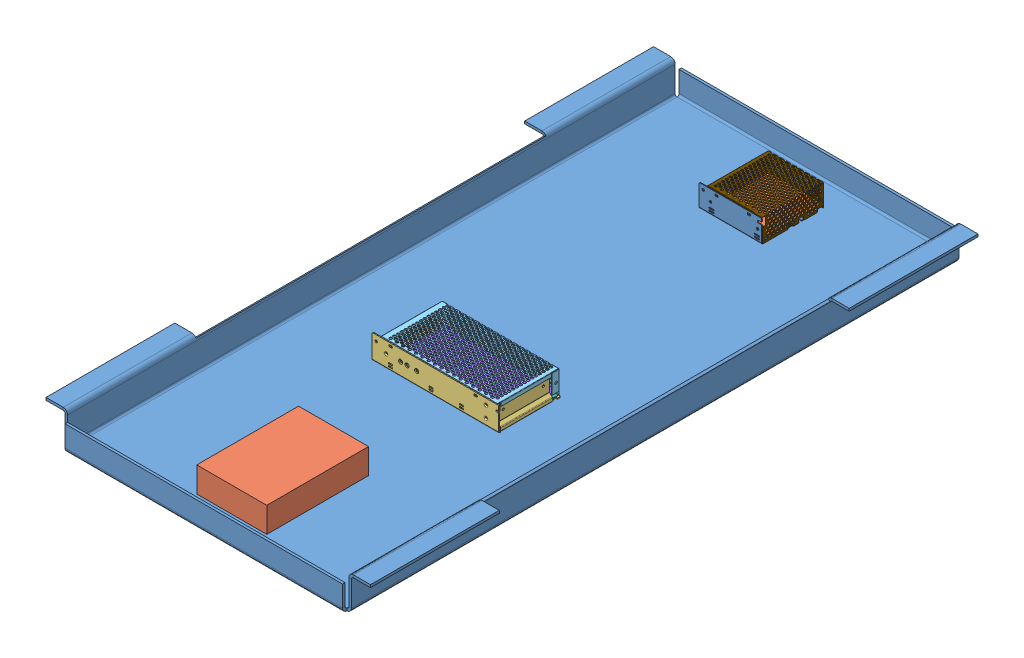
SolidWorks assembly electric_box, configuration Default. Lengths in mm.
Overall size (510 54 969).
30 component instances, 20 part files, 10 mates.
Components (placement in the parent):
- 00-P-PT0154-3-1: 00-P-PT0154-3 [Default] at (0 -9.104 0) size (510 54 969)
- panda_mockup-1: panda_mockup [Default] at (0 -1.504 360.5) x (1 0 0) z (0 -1 0) size (110 160 39.6)
- SD-100C-12-1: SD-100C-12 [Default] at (0 -3.604 71.625) size (199.09 37.75 98.27)
  - SD-100C-12.stp-1: SD-100C-12.stp [Default] at origin size (199.09 37.75 98.27)
    - SD-100-20201028.stp.stp-1: SD-100-20201028.stp.stp [Default] at origin size (199.09 37.75 98.27)
      - SD-100_STP.ASM.stp-1: SD-100_STP.ASM.stp [Default] at origin size (199.09 37.75 98.27)
        - SD-100_1_ASM.ASM.stp-1: SD-100_1_ASM.ASM.stp [Default] at origin size (199 37.75 98.27)
          - 902-D-80_ASM.ASM.stp-1: 902-D-80_ASM.ASM.stp [Default] at origin size (199 37.75 97.75)
            - 902-D-119_PRT.PRT.stp-1: 902-D-119_PRT.PRT.stp [Default] at origin size (199 37.75 97.75)
            - NUT_PRT.PRT.stp-1: NUT_PRT.PRT.stp [Default] at (-111.528 -1.5 -40.7894) x (-1 0 0) z (0 1 0) size (8 6.93 6)
          - 902-T_PRT.PRT.stp-1: 902-T_PRT.PRT.stp [Default] at (96.5 36.1 -49.375) x (-1 0 0) z (0 0 -1) size (195.5 36.02 96.52)
          - MYLAR_PRT.PRT.stp-1: MYLAR_PRT.PRT.stp [Default] at (79.2081 1.5 46.5396) x (-1 0 0) z (0 -1 0) size (197 95 0.5)
          - HS2_PRT.PRT.stp-1: HS2_PRT.PRT.stp [Default] at (-64.5 -80.2586 -88.3567) x (0 0 1) z (-1 0 0) size (6.4 28 55)
          - PCB_PRT.PRT.stp-1: PCB_PRT.PRT.stp [Default] at (-189.5595 4.5 45.0362) x (1 0 0) z (0 1 0) size (194 95 1.6)
        - T44-BS1R05370120201023_STP.ASM.stp-1: T44-BS1R05370120201023_STP.ASM.stp [Default] at (-82.3888 6.1 -32.875) x (0 0 1) z (0 1 0) size (69.8 18 18.8)
          - 6_PRT.PRT.stp-1: 6_PRT.PRT.stp [Default] at origin size (7.51 7.5 3.96)
          - 2_PRT.PRT.stp-1: 2_PRT.PRT.stp [Default] at origin size (7.5 7.5 3.96)
          - 3_PRT.PRT.stp-1: 3_PRT.PRT.stp [Default] at origin size (7.51 7.5 3.96)
          - 4_PRT.PRT.stp-1: 4_PRT.PRT.stp [Default] at (0 0.8 0) size (69.8 18 18.8)
          - 5_PRT.PRT.stp-1: 5_PRT.PRT.stp [Default] at origin size (7.51 7.5 3.96)
          - 6_PRT_1.PRT.stp-1: 6_PRT_1.PRT.stp [Default] at (9.5 0 0) size (7.51 7.5 3.96)
          - 6_PRT_1_1.PRT.stp-1: 6_PRT_1_1.PRT.stp [Default] at (19 0 0) size (7.51 7.5 3.96)
          - 6_PRT_1_1_1.PRT.stp-1: 6_PRT_1_1_1.PRT.stp [Default] at (28.5 0 0) size (7.51 7.5 3.96)
- SD-25C-12-1: SD-25C-12 [Default] at (266.6665 2.696 -156.4754) x (1 0 0) z (0 1 0) size (99.05 97.03 36.06)
  - SD-25C-12.stp-1: SD-25C-12.stp [Default] at origin size (99.05 97.03 36.06)
    - RS-50_ASM_15.ASM.stp-1: RS-50_ASM_15.ASM.stp [Default] at origin size (99.05 97.03 36.06)
      - TN1_2.PRT.stp-1: TN1_2.PRT.stp [Default] at (-301.0065 335.8998 37.1723) x (0 0 -1) z (-1 0 0) size (15.25 49.25 14.66)
      - RS-50-CASE-T_21.PRT.stp-1: RS-50-CASE-T_21.PRT.stp [Default] at (0 1.5 1) size (97.05 96.6 36.06)
      - RS-50-CASE-D_28.PRT.stp-1: RS-50-CASE-D_28.PRT.stp [Default] at (-0.5 0.5 0) size (98.5 97 35)
      - RS-50-PCB_2.PRT.stp-1: RS-50-PCB_2.PRT.stp [Default] at (0 -0.6 -0.2033) size (98 95 1.6)
Mates (geometry in assembly coordinates):
- Coincidente1: coincident: point of 00-P-PT0154-3-1
- Coincidente2: coincident: plane of 00-P-PT0154-3-1 through (-225 -5.104 477.5) normal (0 1 0); plane of panda_mockup-1 through (0 -5.104 360.5) normal (0 -1 0)
- Distanza1: distance = 40 mm anti-aligned: plane of panda_mockup-1 through (-55 34.496 440.5) normal (0 0 1); plane of 00-P-PT0154-3-1 through (0 -9.104 480.5) normal (0 0 -1)
- Larghezza1: width anti-aligned: plane of 00-P-PT0154-3-1 through (-221 -9.104 477.5) normal (1 0 0); plane of panda_mockup-1 through (221 -9.104 477.5) normal (-1 0 0); plane of 00-P-PT0154-3-1 through (-55 34.496 440.5) normal (-1 0 0); plane of panda_mockup-1 through (55 34.496 440.5) normal (1 0 0)
- Coincidente5: coincident anti-aligned: plane of 00-P-PT0154-3-1 through (-225 -5.104 477.5) normal (0 1 0); plane of SD-100C-12-1/SD-100C-12.stp-1/SD-100-20201028.stp.stp-1/SD-100_STP.ASM.stp-1/SD-100_1_ASM.ASM.stp-1/902-D-80_ASM.ASM.stp-1/902-D-119_PRT.PRT.stp-1 through (0 -5.104 71.8131) normal (0 -1 0)
- Coincidente6: coincident: plane of 00-P-PT0154-3-1 through (-225 -5.104 477.5) normal (0 1 0); plane of SD-25C-12-1/SD-25C-12.stp-1/RS-50_ASM_15.ASM.stp-1/RS-50-CASE-D_28.PRT.stp-1 through (101.7147 -5.104 -373.2505) normal (0 -1 0)
- Distanza2: distance = 40 mm: plane of 00-P-PT0154-3-1 through (0 -9.104 -480.5) normal (0 0 1); plane of SD-25C-12-1/SD-25C-12.stp-1/RS-50_ASM_15.ASM.stp-1/RS-50-CASE-T_21.PRT.stp-1 through (-37.5 -2.604 -440.5) normal (0 0 -1)
- Larghezza2: width anti-aligned: plane of 00-P-PT0154-3-1 through (221 -9.104 477.5) normal (-1 0 0); plane of SD-25C-12-1/SD-25C-12.stp-1/RS-50_ASM_15.ASM.stp-1/RS-50-CASE-T_21.PRT.stp-1 through (-221 -9.104 477.5) normal (1 0 0); plane of 00-P-PT0154-3-1 through (53.4714 -2.3142 -392.1132) normal (1 0 0); plane of SD-25C-12-1/SD-25C-12.stp-1/RS-50_ASM_15.ASM.stp-1/RS-50-CASE-D_28.PRT.stp-1 through (-45.5286 3.5913 -359.8228) normal (-1 0 0)
- Larghezza3: width anti-aligned: plane of 00-P-PT0154-3-1 through (-221 -9.104 477.5) normal (1 0 0); plane of SD-100C-12-1/SD-100C-12.stp-1/SD-100-20201028.stp.stp-1/SD-100_STP.ASM.stp-1/SD-100_1_ASM.ASM.stp-1/902-D-80_ASM.ASM.stp-1/902-D-119_PRT.PRT.stp-1 through (221 -9.104 477.5) normal (-1 0 0); plane of 00-P-PT0154-3-1 through (-99.5 -4.354 71.8131) normal (-1 0 0); plane of SD-100C-12-1/SD-100C-12.stp-1/SD-100-20201028.stp.stp-1/SD-100_STP.ASM.stp-1/SD-100_1_ASM.ASM.stp-1/902-D-80_ASM.ASM.stp-1/902-D-119_PRT.PRT.stp-1 through (99.5 -5.104 22.9381) normal (1 0 0)
- Distanza3: distance = 160 mm anti-aligned: plane of SD-100C-12-1/SD-100C-12.stp-1/SD-100-20201028.stp.stp-1/SD-100_STP.ASM.stp-1/SD-100_1_ASM.ASM.stp-1/902-D-80_ASM.ASM.stp-1/902-D-119_PRT.PRT.stp-1 through (99.5 -5.104 120.5) normal (0 0 1); plane of panda_mockup-1 through (-55 34.496 280.5) normal (0 0 -1)
